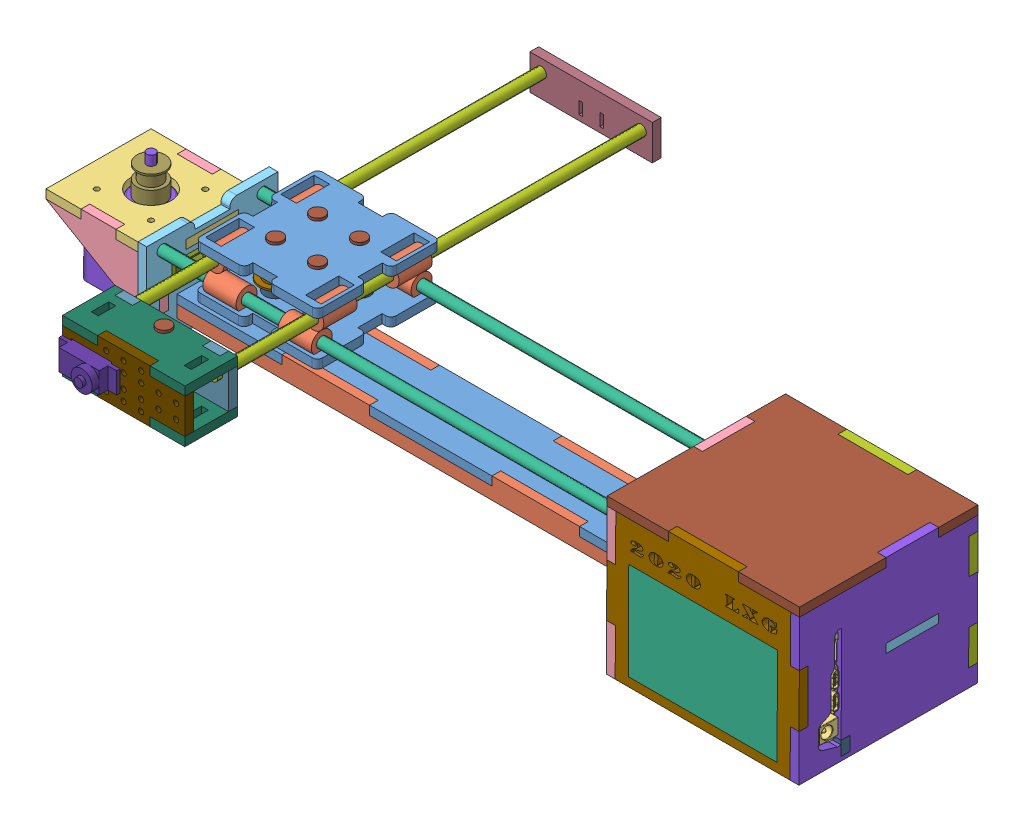
SolidWorks assembly 合V1.0, configuration 默认. Lengths in mm.
Overall size (465 88.44 285.26).
63 component instances, 29 part files, 128 mates.
Components (placement in the parent):
- 中心同步块-1: 中心同步块 [默认] at (-116.6311 89.0687 -129.5565) x (0 0.004224 0.999991) z (0 -0.999991 0.004224) size (70 70 5)
- 中心同步块-2: 中心同步块 [默认] at (-186.6311 114.1177 -129.6623) x (1 0 0) z (0 -0.999991 0.004224) size (70 70 5)
- 直线轴承 内径6MMx外径12MMx长度19MM-1: 直线轴承 内径6MMx外径12MMx长度19MM [默认] at (-139.6311 93.3617 -66.024) x (0 0.863153 -0.504943) z (1 0 0) size (13.89 12 19)
- 直线轴承 内径6MMx外径12MMx长度19MM-2: 直线轴承 内径6MMx外径12MMx长度19MM [默认] at (-180.1811 105.1903 -106.6244) x (0.934679 0.35549 -0.001501) z (0 -0.004224 -0.999991) size (13.89 12 19)
- 长端无控制器端电机座上-1: 长端无控制器端电机座上 [默认] at (-216.7731 91.6144 -124.5672) x (0 0.004224 0.999991) z (0 -0.999991 0.004224) size (60 65 5)
- 长端无控制器端电机座侧面-1: 长端无控制器端电机座侧面 [默认] at (-216.7731 51.8471 -69.3987) x (1 0 0) z (0 0.004224 0.999991) size (65 40 5)
- 长端无控制器端电机座侧面-2: 长端无控制器端电机座侧面 [默认] at (-216.7731 51.6148 -124.3982) x (1 0 0) z (0 0.004224 0.999991) size (65 40 5)
- 长端无控制器端-1: 长端无控制器端 [默认] at (-216.7731 46.0726 -134.3749) x (0 -0.004224 -0.999991) z (1 0 0) size (80 53 5)
- 直线轴承 内径6MMx外径12MMx长度19MM-3: 直线轴承 内径6MMx外径12MMx长度19MM [默认] at (-182.6311 93.1205 -123.1235) x (0 0.999978 -0.006661) z (1 0 0) size (13.89 12 19)
- 直线轴承 内径6MMx外径12MMx长度19MM-4: 直线轴承 内径6MMx外径12MMx长度19MM [默认] at (-182.6311 93.3617 -66.024) x (0 0.949917 -0.312502) z (1 0 0) size (13.89 12 19)
- 直线轴承 内径6MMx外径12MMx长度19MM-5: 直线轴承 内径6MMx外径12MMx长度19MM [默认] at (-139.6311 93.1205 -123.1235) x (0 0.946256 0.323419) z (1 0 0) size (13.89 12 19)
- 直线轴承 内径6MMx外径12MMx长度19MM-6: 直线轴承 内径6MMx外径12MMx长度19MM [默认] at (-123.0811 105.2917 -82.6246) x (-0.725747 -0.687956 0.002906) z (0 0.004224 0.999991) size (13.89 12 19)
- 直线轴承 内径6MMx外径12MMx长度19MM-7: 直线轴承 内径6MMx外径12MMx长度19MM [默认] at (-123.0811 105.1903 -106.6244) x (1 0 0) z (0 -0.004224 -0.999991) size (13.89 12 19)
- 直线轴承 内径6MMx外径12MMx长度19MM-8: 直线轴承 内径6MMx外径12MMx长度19MM [默认] at (-180.1811 105.3719 -63.6247) x (1 0 0) z (0 -0.004224 -0.999991) size (13.89 12 19)
- 光杆300MMx6MM-1: 光杆300MMx6MM [默认] at (83.2269 93.3617 -66.024) x (0 0 1) z (-1 0 0) size (6 6 300)
- 光杆300MMx6MM-2: 光杆300MMx6MM [默认] at (83.2269 93.1205 -123.1235) x (0 0 1) z (-1 0 0) size (6 6 300)
- 光杆250MMx6MM-3: 光杆250MMx6MM [默认] at (-180.1811 104.5595 -255.9817) x (-0.383385 -0.92358 0.003901) z (0 0.004224 0.999991) size (6 6 250)
- 光杆250MMx6MM-4: 光杆250MMx6MM [默认] at (-123.0811 104.5595 -255.9817) x (0.573262 0.819365 -0.003461) z (0 0.004224 0.999991) size (6 6 250)
- 42步进电机-1: 42步进电机 [默认] at (-267.9231 86.8305 -73.3965) x (0 -0.999991 0.004224) z (0 0.004224 0.999991) size (61.5 49.3 42.3)
- 42步进电机-2: 42步进电机 [默认] at (134.3769 86.6518 -115.6961) x (0 -0.999991 0.004224) z (0 -0.004224 -0.999991) size (61.5 49.3 42.3)
- 2GT_20齿同步轮 H型皮带轮 带宽6MM 内孔5MM-1: 2GT_20齿同步轮 H型皮带轮 带宽6MM 内孔5MM [默认] at (-163.6311 102.4606 -82.6126) x (0.996537 0.000351 0.08315) z (0 -0.999991 0.004224) size (18 18 8.5)
- 内径5MM 外径10MM 厚度6MM隔离柱-1: 内径5MM 外径10MM 厚度6MM隔离柱 [默认] at (-163.6311 103.4606 -82.6168) x (1 0 0) z (0 0.004224 0.999991) size (12 6 12)
- M5x35MM螺丝-1: M5x35MM螺丝 [默认] at (-163.6311 79.3165 -82.5149) x (1 0 0) z (0 0.004224 0.999991) size (8.05 36.5 8.05)
- 内径5MM 外径10MM 厚度6MM隔离柱-2: 内径5MM 外径10MM 厚度6MM隔离柱 [默认] at (-163.6311 88.9607 -82.5556) x (1 0 0) z (0 0.004224 0.999991) size (12 6 12)
- 内径5MM 外径10MM 厚度6MM隔离柱-3: 内径5MM 外径10MM 厚度6MM隔离柱 [默认] at (-139.6311 107.2087 -82.6327) x (0.081874 0.004209 0.996634) z (-0.996643 0.000346 0.081873) size (12 6 12)
- 2GT_20齿同步轮 H型皮带轮 带宽6MM 内孔5MM-2: 2GT_20齿同步轮 H型皮带轮 带宽6MM 内孔5MM [默认] at (-139.6311 106.2087 -82.6284) x (1 0 0) z (0 -0.999991 0.004224) size (18 18 8.5)
- 内径5MM 外径10MM 厚度6MM隔离柱-4: 内径5MM 外径10MM 厚度6MM隔离柱 [默认] at (-139.6311 92.7089 -82.5714) x (0.998633 -0.000221 -0.052265) z (0.052266 0.004218 0.998624) size (12 6 12)
- M5x35MM螺丝-2: M5x35MM螺丝 [默认] at (-139.6311 79.3165 -82.5149) x (1 0 0) z (0 0.004224 0.999991) size (8.05 36.5 8.05)
- 同步轮2GT带宽6MM 20齿内孔5MM-1: 同步轮2GT带宽6MM 20齿内孔5MM [默认] at (-246.7731 88.7411 -94.5548) x (0.755628 0.002766 0.654995) z (-0.655001 0.003191 0.755621) size (16 16 16)
- 内径5MM 外径10MM 厚度6MM隔离柱-5: 内径5MM 外径10MM 厚度6MM隔离柱 [默认] at (-163.6311 89.4064 -106.5577) x (1 0 0) z (0 0.004224 0.999991) size (12 6 12)
- M5x35MM螺丝-3: M5x35MM螺丝 [默认] at (-163.6311 79.2152 -106.5146) x (1 0 0) z (0 0.004224 0.999991) size (8.05 36.5 8.05)
- 2GT_20齿同步轮 H型皮带轮 带宽6MM 内孔5MM-3: 2GT_20齿同步轮 H型皮带轮 带宽6MM 内孔5MM [默认] at (-163.6311 102.9063 -106.6147) x (1 0 0) z (0 -0.999991 0.004224) size (18 18 8.5)
- 内径5MM 外径10MM 厚度6MM隔离柱-6: 内径5MM 外径10MM 厚度6MM隔离柱 [默认] at (-163.6311 103.9063 -106.6189) x (0.113852 0.004196 0.993489) z (-0.993498 0.000481 0.113851) size (12 6 12)
- 内径5MM 外径10MM 厚度6MM隔离柱-7: 内径5MM 外径10MM 厚度6MM隔离柱 [默认] at (-139.6311 89.407 -106.5577) x (0.997535 -0.000296 -0.070166) z (0.070166 0.004213 0.997526) size (12 6 12)
- M5x35MM螺丝-4: M5x35MM螺丝 [默认] at (-139.6311 79.2152 -106.5146) x (1 0 0) z (0 0.004224 0.999991) size (8.05 36.5 8.05)
- 2GT_20齿同步轮 H型皮带轮 带宽6MM 内孔5MM-4: 2GT_20齿同步轮 H型皮带轮 带宽6MM 内孔5MM [默认] at (-139.6311 102.9069 -106.6147) x (1 0 0) z (0 -0.999991 0.004224) size (18 18 8.5)
- 内径5MM 外径10MM 厚度6MM隔离柱-8: 内径5MM 外径10MM 厚度6MM隔离柱 [默认] at (-139.6311 103.9069 -106.6189) x (0.631814 0.003274 0.775113) z (-0.77512 0.002669 0.631809) size (12 6 12)
- 短端结扎-1: 短端结扎 [默认] at (-151.6311 101.5595 -255.9691) x (1 0 0) z (0 -0.999991 0.004224) size (70 5 20)
- 短端抬笔侧-1: 短端抬笔侧 [默认] at (-186.6311 89.5825 -13.7378) x (1 0 0) z (0 -0.999991 0.004224) size (20 5 30)
- 短端抬笔上-1: 短端抬笔上 [默认] at (-186.6311 109.709 16.1774) x (1 0 0) z (0 0.004224 0.999991) size (70 5 30)
- 短端抬笔侧-2: 短端抬笔侧 [默认] at (-116.6311 89.6036 -8.7379) x (-1 0 0) z (0 -0.999991 0.004224) size (20 5 30)
- 短端抬笔上-2: 短端抬笔上 [默认] at (-116.6311 89.7092 16.2619) x (-1 0 0) z (0 0.004224 0.999991) size (70 5 30)
- M5x35MM螺丝-5: M5x35MM螺丝 [默认] at (-151.6311 79.6121 -6.6957) x (-0.916947 0.001685 0.399005) z (-0.399008 -0.003873 -0.916939) size (8.05 36.5 8.05)
- 内径5MM 外径10MM 厚度6MM隔离柱-9: 内径5MM 外径10MM 厚度6MM隔离柱 [默认] at (-151.6311 89.2051 -6.7362) x (0.998633 -0.000221 -0.052265) z (0.052266 0.004218 0.998624) size (12 6 12)
- 2GT_20齿同步轮 H型皮带轮 带宽6MM 内孔5MM-5: 2GT_20齿同步轮 H型皮带轮 带宽6MM 内孔5MM [默认] at (-151.6311 102.705 -6.7932) x (1 0 0) z (0 -0.999991 0.004224) size (18 18 8.5)
- 内径5MM 外径10MM 厚度6MM隔离柱-10: 内径5MM 外径10MM 厚度6MM隔离柱 [默认] at (-151.6311 103.705 -6.7974) x (0.928854 0.001565 0.370443) z (-0.370447 0.003923 0.928845) size (12 6 12)
- 限位开关-1: 限位开关 [默认] at (-225.4635 76.6652 -112.5039) x (0 0.004224 0.999991) z (-1 0 0) size (41 7.3 21.5)
- SG90舵机-1: SG90舵机 [默认] at (-181.6311 92.7091 1.2491) x (1 0 0) z (0 -0.999991 0.004224) size (33 28 12.05)
- 短端抬笔前-1: 短端抬笔前 [默认] at (-186.6311 89.6881 11.2619) x (1 0 0) z (0 -0.999991 0.004224) size (70 5 30)
- 底部大横-1: 底部大横 [默认] at (-211.7731 62.1569 -114.4427) x (0 0.004224 0.999991) z (-1 0 0) size (40 5 300)
- 底部大横竖-1: 底部大横竖 [默认] at (-216.7731 55.3048 -79.4134) x (1 0 0) z (0 -0.999991 0.004224) size (300 5 12)
- 底部大横竖-2: 底部大横竖 [默认] at (-216.7731 55.157 -114.4131) x (1 0 0) z (0 -0.999991 0.004224) size (300 5 12)
- 限位开关-2: 限位开关 [默认] at (-145.6311 84.6501 2.2831) x (-1 0 0) z (0 0.004224 0.999991) size (41 7.3 21.5)
- ArtistV1-1: ArtistV1 [默认] at (88.2308 47.6829 -53.5734) x (1 0 0) z (0 0.004224 0.999991) size (99.16 80.01 19.91)
- 长端控制器端-1: 长端控制器端 [默认] at (83.2269 46.4105 -54.3756) x (0 0.004224 0.999991) z (-1 0 0) size (102 88 5)
- 长端控制器端电机座上-1: 长端控制器端电机座上 [默认] at (83.2269 86.6144 -124.5461) x (0 0.004224 0.999991) z (0 0.999991 -0.004224) size (62.5 110 5)
- 同步轮2GT带宽6MM 20齿内孔5MM-2: 同步轮2GT带宽6MM 20齿内孔5MM [默认] at (113.2269 92.1104 -94.569) x (0.99941 -0.000145 -0.034342) z (0.034343 0.004221 0.999401) size (16 16 16)
- 3.5寸LCD-1: 3.5寸LCD [默认] at (37.2293 48.6901 -33.4851) x (1 0 0) z (0 0.004224 0.999991) size (85 55.5 3.6)
- 长端控制器端后-1: 长端控制器端后 [默认] at (83.2269 46.0831 -131.8749) x (1 0 0) z (0 0.004224 0.999991) size (110 88 5)
- 长端控制器端右-1: 长端控制器端右 [默认] at (188.2269 76.8541 -60.2099) x (-1 0 0) z (0 -0.004224 -0.999991) size (5 88 102)
- 长端控制器端前-1: 长端控制器端前 [默认] at (83.2269 46.4928 -34.8758) x (1 0 0) z (0 0.004224 0.999991) size (110 88 5)
- 长端控制器端pcb座-1: 长端控制器端pcb座 [默认] at (157.8191 48.8702 -53.9544) x (0 -0.004224 -0.999991) z (1 0 0) size (5 20 110)
- 长端控制器端上-1: 长端控制器端上 [默认] at (78.2269 129.5132 -30.2264) x (1 0 0) z (0 0.004224 0.999991) size (110 5 102)
Mates (geometry in assembly coordinates):
- 重合1: coincident aligned: line of 长端无控制器端电机座上-1 through (-211.7731 91.6778 -109.5673) axis (0 0.004224 0.999991); line of 长端无控制器端-1 through (-211.7731 91.6778 -109.5673) axis (0 0.004224 0.999991)
- 重合2: coincident anti-aligned: line of 长端无控制器端电机座上-1 through (-211.7731 86.8045 -79.5465) axis (0 0.999991 -0.004224); line of 长端无控制器端-1 through (-211.7731 91.8045 -79.5676) axis (0 -0.999991 0.004224)
- 重合3: coincident aligned: line of 长端无控制器端电机座上-1 through (-236.7731 91.8467 -69.5677) axis (-1 0 0); line of 长端无控制器端电机座侧面-1 through (-236.7731 91.8467 -69.5677) axis (-1 0 0)
- 重合4: coincident aligned: line of 长端无控制器端电机座上-1 through (-236.7731 91.8678 -64.5677) axis (0 -0.004224 -0.999991); line of 长端无控制器端电机座侧面-1 through (-236.7731 91.8678 -64.5677) axis (0 -0.004224 -0.999991)
- 重合5: coincident anti-aligned: line of 长端无控制器端电机座上-1 through (-256.7731 91.6355 -119.5672) axis (1 0 0); line of 长端无控制器端电机座侧面-2 through (-236.7731 91.6355 -119.5672) axis (-1 0 0)
- 重合6: coincident aligned: line of 长端无控制器端电机座上-1 through (-236.7731 91.6355 -119.5672) axis (0 -0.004224 -0.999991); line of 长端无控制器端电机座侧面-2 through (-236.7731 91.6355 -119.5672) axis (0 -0.004224 -0.999991)
- 重合13: coincident anti-aligned: circle of 长端无控制器端电机座上-1; circle of 42步进电机-1
- 同心1: concentric anti-aligned: cylinder of 长端无控制器端-1 through (-211.7731 93.3617 -66.024) axis (-1 0 0) radius 3; cylinder of 光杆300MMx6MM-1 through (-216.7731 93.3617 -66.024) axis (1 0 0) radius 3
- 同心2: concentric anti-aligned: cylinder of 长端无控制器端-1 through (-211.7731 93.1205 -123.1235) axis (-1 0 0) radius 3; cylinder of 光杆300MMx6MM-2 through (-216.7731 93.1205 -123.1235) axis (1 0 0) radius 3
- 重合17: coincident anti-aligned: circle of 长端无控制器端-1; circle of 光杆300MMx6MM-1
- 重合18: coincident anti-aligned: circle of 长端无控制器端-1; circle of 光杆300MMx6MM-2
- 同心6: concentric anti-aligned: cylinder of 直线轴承 内径6MMx外径12MMx长度19MM-4 through (-163.6311 93.3617 -66.024) axis (-1 0 0) radius 3; cylinder of 光杆300MMx6MM-1 through (-216.7731 93.3617 -66.024) axis (1 0 0) radius 3
- 同心7: concentric anti-aligned: cylinder of 直线轴承 内径6MMx外径12MMx长度19MM-1 through (-120.6311 93.3617 -66.024) axis (-1 0 0) radius 3; cylinder of 光杆300MMx6MM-1 through (-216.7731 93.3617 -66.024) axis (1 0 0) radius 3
- 同心8: concentric anti-aligned: cylinder of 直线轴承 内径6MMx外径12MMx长度19MM-3 through (-163.6311 93.1205 -123.1235) axis (-1 0 0) radius 3; cylinder of 光杆300MMx6MM-2 through (-216.7731 93.1205 -123.1235) axis (1 0 0) radius 3
- 同心9: concentric anti-aligned: cylinder of 直线轴承 内径6MMx外径12MMx长度19MM-5 through (-120.6311 93.1205 -123.1235) axis (-1 0 0) radius 3; cylinder of 光杆300MMx6MM-2 through (-216.7731 93.1205 -123.1235) axis (1 0 0) radius 3
- 同心10: concentric anti-aligned: cylinder of 2GT_20齿同步轮 H型皮带轮 带宽6MM 内孔5MM-1 through (-163.6311 95.9606 -82.5852) axis (0 0.999991 -0.004224) radius 2.5; cylinder of M5x35MM螺丝-1 through (-163.6311 114.3162 -82.6627) axis (0 -0.999991 0.004224) radius 2.5
- 同心11: concentric aligned: cylinder of 内径5MM 外径10MM 厚度6MM隔离柱-1 through (-163.6311 109.4605 -82.6422) axis (0 -0.999991 0.004224) radius 3; cylinder of M5x35MM螺丝-1 through (-163.6311 114.3162 -82.6627) axis (0 -0.999991 0.004224) radius 2.5
- 同心12: concentric aligned: cylinder of M5x35MM螺丝-1 through (-163.6311 114.3162 -82.6627) axis (0 -0.999991 0.004224) radius 2.5; cylinder of 内径5MM 外径10MM 厚度6MM隔离柱-2 through (-163.6311 94.9607 -82.5809) axis (0 -0.999991 0.004224) radius 3
- 同心13: concentric aligned: cylinder of 内径5MM 外径10MM 厚度6MM隔离柱-3 through (-139.6311 113.2087 -82.658) axis (0 -0.999991 0.004224) radius 3; cylinder of M5x35MM螺丝-2 through (-139.6311 114.3162 -82.6627) axis (0 -0.999991 0.004224) radius 2.5
- 同心14: concentric aligned: cylinder of 内径5MM 外径10MM 厚度6MM隔离柱-4 through (-139.6311 98.7088 -82.5968) axis (0 -0.999991 0.004224) radius 3; cylinder of M5x35MM螺丝-2 through (-139.6311 114.3162 -82.6627) axis (0 -0.999991 0.004224) radius 2.5
- 同心15: concentric anti-aligned: cylinder of 2GT_20齿同步轮 H型皮带轮 带宽6MM 内孔5MM-2 through (-139.6311 99.7088 -82.601) axis (0 0.999991 -0.004224) radius 2.5; cylinder of M5x35MM螺丝-2 through (-139.6311 114.3162 -82.6627) axis (0 -0.999991 0.004224) radius 2.5
- 重合19: coincident aligned: plane of 2GT_20齿同步轮 H型皮带轮 带宽6MM 内孔5MM-1 through (-163.6311 103.4606 -82.6168) normal (0 0.999991 -0.004224); circle of 内径5MM 外径10MM 厚度6MM隔离柱-1
- 重合20: coincident anti-aligned: plane of 2GT_20齿同步轮 H型皮带轮 带宽6MM 内孔5MM-1 through (-163.6311 94.9607 -82.5809) normal (0 -0.999991 0.004224); plane of 内径5MM 外径10MM 厚度6MM隔离柱-2 through (-163.6311 94.9607 -82.5809) normal (0 0.999991 -0.004224)
- 同心16: concentric aligned: cylinder of 中心同步块-1 through (-163.6311 84.2673 -82.5358) axis (0 0.999991 -0.004224) radius 2.5; cylinder of 中心同步块-2 through (-163.6311 109.3163 -82.6416) axis (0 0.999991 -0.004224) radius 2.5
- 同心17: concentric aligned: cylinder of 中心同步块-1 through (-139.6311 84.2673 -82.5358) axis (0 0.999991 -0.004224) radius 2.5; cylinder of 中心同步块-2 through (-139.6311 109.3163 -82.6416) axis (0 0.999991 -0.004224) radius 2.5
- 同心18: concentric anti-aligned: cylinder of 中心同步块-2 through (-163.6311 109.3163 -82.6416) axis (0 0.999991 -0.004224) radius 2.5; cylinder of M5x35MM螺丝-1 through (-163.6311 114.3162 -82.6627) axis (0 -0.999991 0.004224) radius 2.5
- 重合21: coincident anti-aligned: plane of 中心同步块-2 through (-161.6311 114.1304 -126.6623) normal (0 0.999991 -0.004224); plane of M5x35MM螺丝-1 through (-163.6311 114.3162 -82.6627) normal (0 -0.999991 0.004224)
- 相切2: tangent: line of 中心同步块-1 through (-163.6311 89.1147 -118.6566) axis (-1 0 0); cylinder of 直线轴承 内径6MMx外径12MMx长度19MM-3 through (-163.6311 93.1205 -123.1235) axis (-1 0 0) radius 6
- 重合24: coincident: line of 中心同步块-1 through (-182.6311 89.3559 -61.5571) axis (0 -0.004224 -0.999991); plane of 直线轴承 内径6MMx外径12MMx长度19MM-4 through (-182.6311 93.3617 -66.024) normal (-1 0 0)
- 重合25: coincident: line of 中心同步块-1 through (-163.6311 89.3559 -61.5571) axis (-1 0 0); cylinder of 直线轴承 内径6MMx外径12MMx长度19MM-4 through (-163.6311 93.3617 -66.024) axis (-1 0 0) radius 6
- 重合26: coincident: line of 中心同步块-1 through (-182.6311 89.1147 -118.6566) axis (0 -0.004224 -0.999991); plane of 直线轴承 内径6MMx外径12MMx长度19MM-3 through (-182.6311 93.1205 -123.1235) normal (-1 0 0)
- 重合27: coincident: line of 中心同步块-1 through (-182.6311 89.3183 -70.457) axis (1 0 0); cylinder of 直线轴承 内径6MMx外径12MMx长度19MM-4 through (-163.6311 93.3617 -66.024) axis (-1 0 0) radius 6
- 重合28: coincident: line of 中心同步块-1 through (-120.6311 89.3183 -70.457) axis (0 0.004224 0.999991); plane of 直线轴承 内径6MMx外径12MMx长度19MM-1 through (-120.6311 93.3617 -66.024) normal (1 0 0)
- 重合29: coincident: line of 中心同步块-1 through (-120.6311 89.0771 -127.5565) axis (0 0.004224 0.999991); plane of 直线轴承 内径6MMx外径12MMx长度19MM-5 through (-120.6311 93.1205 -123.1235) normal (1 0 0)
- 重合30: coincident: line of 中心同步块-2 through (-184.6311 109.3965 -63.6417) axis (0 -0.004224 -0.999991); cylinder of 直线轴承 内径6MMx外径12MMx长度19MM-8 through (-180.1811 105.2917 -82.6246) axis (0 0.004224 0.999991) radius 6
- 重合31: coincident: line of 中心同步块-2 through (-175.7311 109.3163 -82.6416) axis (0 0.004224 0.999991); cylinder of 直线轴承 内径6MMx外径12MMx长度19MM-8 through (-180.1811 105.2917 -82.6246) axis (0 0.004224 0.999991) radius 6
- 重合32: coincident anti-aligned: plane of 中心同步块-2 through (-184.6311 109.3163 -82.6416) normal (0 0.004224 0.999991); plane of 直线轴承 内径6MMx外径12MMx长度19MM-8 through (-180.1811 105.2917 -82.6246) normal (0 -0.004224 -0.999991)
- 相切3: tangent anti-aligned: cylinder of 直线轴承 内径6MMx外径12MMx长度19MM-4 through (-163.6311 93.3617 -66.024) axis (-1 0 0) radius 6; cylinder of 直线轴承 内径6MMx外径12MMx长度19MM-8 through (-180.1811 105.2917 -82.6246) axis (0 0.004224 0.999991) radius 6
- 同心20: concentric anti-aligned: cylinder of 直线轴承 内径6MMx外径12MMx长度19MM-8 through (-180.1811 105.2917 -82.6246) axis (0 0.004224 0.999991) radius 3; cylinder of 光杆250MMx6MM-3 through (-180.1811 105.6154 -5.984) axis (0 -0.004224 -0.999991) radius 3
- 重合33: coincident anti-aligned: plane of 中心同步块-2 through (-127.5311 109.3163 -82.6416) normal (0 0.004224 0.999991); plane of 直线轴承 内径6MMx外径12MMx长度19MM-6 through (-123.0811 105.2917 -82.6246) normal (0 -0.004224 -0.999991)
- 重合36: coincident: line of 中心同步块-2 through (-118.6311 109.3163 -82.6416) axis (0 0.004224 0.999991); cylinder of 直线轴承 内径6MMx外径12MMx长度19MM-6 through (-123.0811 105.3719 -63.6247) axis (0 -0.004224 -0.999991) radius 6
- 重合37: coincident: line of 中心同步块-2 through (-127.5311 109.3965 -63.6417) axis (0 -0.004224 -0.999991); cylinder of 直线轴承 内径6MMx外径12MMx长度19MM-6 through (-123.0811 105.3719 -63.6247) axis (0 -0.004224 -0.999991) radius 6
- 重合38: coincident: line of 中心同步块-2 through (-127.5311 109.2149 -106.6414) axis (0 -0.004224 -0.999991); cylinder of 直线轴承 内径6MMx外径12MMx长度19MM-7 through (-123.0811 105.1101 -125.6242) axis (0 0.004224 0.999991) radius 6
- 重合39: coincident: line of 中心同步块-2 through (-118.6311 109.1346 -125.6412) axis (0 0.004224 0.999991); cylinder of 直线轴承 内径6MMx外径12MMx长度19MM-7 through (-123.0811 105.1101 -125.6242) axis (0 0.004224 0.999991) radius 6
- 重合40: coincident anti-aligned: plane of 中心同步块-2 through (-127.5311 109.1346 -125.6412) normal (0 0.004224 0.999991); plane of 直线轴承 内径6MMx外径12MMx长度19MM-7 through (-123.0811 105.1101 -125.6242) normal (0 -0.004224 -0.999991)
- 重合43: coincident anti-aligned: plane of 中心同步块-2 through (-184.6311 109.2149 -106.6414) normal (0 -0.004224 -0.999991); plane of 直线轴承 内径6MMx外径12MMx长度19MM-2 through (-180.1811 105.1903 -106.6244) normal (0 0.004224 0.999991)
- 相切4: tangent anti-aligned: cylinder of 直线轴承 内径6MMx外径12MMx长度19MM-2 through (-180.1811 105.1101 -125.6242) axis (0 0.004224 0.999991) radius 6; cylinder of 直线轴承 内径6MMx外径12MMx长度19MM-3 through (-163.6311 93.1205 -123.1235) axis (-1 0 0) radius 6
- 同心21: concentric aligned: cylinder of 直线轴承 内径6MMx外径12MMx长度19MM-6 through (-123.0811 105.3719 -63.6247) axis (0 -0.004224 -0.999991) radius 3; cylinder of 光杆250MMx6MM-4 through (-123.0811 105.6154 -5.984) axis (0 -0.004224 -0.999991) radius 3
- 重合44: coincident: line of 中心同步块-2 through (-175.7311 109.1346 -125.6412) axis (0 0.004224 0.999991); cylinder of 直线轴承 内径6MMx外径12MMx长度19MM-2 through (-180.1811 105.1101 -125.6242) axis (0 0.004224 0.999991) radius 6
- 同心22: concentric aligned: cylinder of 42步进电机-1 through (-246.7731 110.2409 -94.6456) axis (0 -0.999991 0.004224) radius 2.5; cylinder of 同步轮2GT带宽6MM 20齿内孔5MM-1 through (-246.7731 96.7411 -94.5886) axis (0 -0.999991 0.004224) radius 2.5
- 重合45: coincident anti-aligned: circle of 长端无控制器端电机座上-1; circle of 42步进电机-1
- 重合46: coincident anti-aligned: plane of 42步进电机-1 through (-246.7731 88.7411 -94.5548) normal (0 0.999991 -0.004224); plane of 同步轮2GT带宽6MM 20齿内孔5MM-1 through (-246.7731 88.7411 -94.5548) normal (0 -0.999991 0.004224)
- 重合47: coincident anti-aligned: plane of 内径5MM 外径10MM 厚度6MM隔离柱-3 through (-139.6311 107.2087 -82.6327) normal (0 -0.999991 0.004224); plane of 2GT_20齿同步轮 H型皮带轮 带宽6MM 内孔5MM-2 through (-139.6311 107.2087 -82.6327) normal (0 0.999991 -0.004224)
- 重合48: coincident anti-aligned: plane of 2GT_20齿同步轮 H型皮带轮 带宽6MM 内孔5MM-2 through (-139.6311 98.7088 -82.5968) normal (0 -0.999991 0.004224); plane of 内径5MM 外径10MM 厚度6MM隔离柱-4 through (-139.6311 98.7088 -82.5968) normal (0 0.999991 -0.004224)
- 同心23: concentric anti-aligned: cylinder of 中心同步块-2 through (-139.6311 109.3163 -82.6416) axis (0 0.999991 -0.004224) radius 2.5; cylinder of M5x35MM螺丝-2 through (-139.6311 114.3162 -82.6627) axis (0 -0.999991 0.004224) radius 2.5
- 同心24: concentric aligned: cylinder of 内径5MM 外径10MM 厚度6MM隔离柱-5 through (-163.6311 95.4064 -106.583) axis (0 -0.999991 0.004224) radius 3; cylinder of M5x35MM螺丝-3 through (-163.6311 114.2148 -106.6625) axis (0 -0.999991 0.004224) radius 2.5
- 同心25: concentric aligned: cylinder of M5x35MM螺丝-3 through (-163.6311 114.2148 -106.6625) axis (0 -0.999991 0.004224) radius 2.5; cylinder of 内径5MM 外径10MM 厚度6MM隔离柱-6 through (-163.6311 109.9063 -106.6443) axis (0 -0.999991 0.004224) radius 3
- 同心26: concentric anti-aligned: cylinder of M5x35MM螺丝-3 through (-163.6311 114.2148 -106.6625) axis (0 -0.999991 0.004224) radius 2.5; cylinder of 2GT_20齿同步轮 H型皮带轮 带宽6MM 内孔5MM-3 through (-163.6311 96.4064 -106.5873) axis (0 0.999991 -0.004224) radius 2.5
- 重合49: coincident anti-aligned: plane of 内径5MM 外径10MM 厚度6MM隔离柱-5 through (-163.6311 95.4064 -106.583) normal (0 0.999991 -0.004224); plane of 2GT_20齿同步轮 H型皮带轮 带宽6MM 内孔5MM-3 through (-163.6311 95.4064 -106.583) normal (0 -0.999991 0.004224)
- 重合50: coincident anti-aligned: plane of 2GT_20齿同步轮 H型皮带轮 带宽6MM 内孔5MM-3 through (-163.6311 103.9063 -106.6189) normal (0 0.999991 -0.004224); plane of 内径5MM 外径10MM 厚度6MM隔离柱-6 through (-163.6311 103.9063 -106.6189) normal (0 -0.999991 0.004224)
- 同心27: concentric aligned: cylinder of 内径5MM 外径10MM 厚度6MM隔离柱-7 through (-139.6311 95.407 -106.583) axis (0 -0.999991 0.004224) radius 3; cylinder of M5x35MM螺丝-4 through (-139.6311 114.2148 -106.6625) axis (0 -0.999991 0.004224) radius 2.5
- 同心28: concentric aligned: cylinder of M5x35MM螺丝-4 through (-139.6311 114.2148 -106.6625) axis (0 -0.999991 0.004224) radius 2.5; cylinder of 内径5MM 外径10MM 厚度6MM隔离柱-8 through (-139.6311 109.9069 -106.6443) axis (0 -0.999991 0.004224) radius 3
- 同心29: concentric anti-aligned: cylinder of M5x35MM螺丝-4 through (-139.6311 114.2148 -106.6625) axis (0 -0.999991 0.004224) radius 2.5; cylinder of 2GT_20齿同步轮 H型皮带轮 带宽6MM 内孔5MM-4 through (-139.6311 96.407 -106.5873) axis (0 0.999991 -0.004224) radius 2.5
- 重合51: coincident anti-aligned: plane of 内径5MM 外径10MM 厚度6MM隔离柱-7 through (-139.6311 95.407 -106.583) normal (0 0.999991 -0.004224); plane of 2GT_20齿同步轮 H型皮带轮 带宽6MM 内孔5MM-4 through (-139.6311 95.407 -106.583) normal (0 -0.999991 0.004224)
- 重合52: coincident anti-aligned: plane of 2GT_20齿同步轮 H型皮带轮 带宽6MM 内孔5MM-4 through (-139.6311 103.9069 -106.6189) normal (0 0.999991 -0.004224); plane of 内径5MM 外径10MM 厚度6MM隔离柱-8 through (-139.6311 103.9069 -106.6189) normal (0 -0.999991 0.004224)
- 同心30: concentric anti-aligned: cylinder of 中心同步块-2 through (-163.6311 109.2149 -106.6414) axis (0 0.999991 -0.004224) radius 2.5; cylinder of M5x35MM螺丝-3 through (-163.6311 114.2148 -106.6625) axis (0 -0.999991 0.004224) radius 2.5
- 同心31: concentric anti-aligned: cylinder of 中心同步块-2 through (-139.6311 109.2149 -106.6414) axis (0 0.999991 -0.004224) radius 2.5; cylinder of M5x35MM螺丝-4 through (-139.6311 114.2148 -106.6625) axis (0 -0.999991 0.004224) radius 2.5
- 重合53: coincident aligned: plane of 中心同步块-2 through (-161.6311 114.1304 -126.6623) normal (0 0.999991 -0.004224); circle of M5x35MM螺丝-2
- 重合54: coincident aligned: plane of 中心同步块-2 through (-161.6311 114.1304 -126.6623) normal (0 0.999991 -0.004224); circle of M5x35MM螺丝-3
- 重合55: coincident aligned: plane of 中心同步块-2 through (-161.6311 114.1304 -126.6623) normal (0 0.999991 -0.004224); circle of M5x35MM螺丝-4
- 同心32: concentric aligned: cylinder of 光杆250MMx6MM-3 through (-180.1811 105.6154 -5.984) axis (0 -0.004224 -0.999991) radius 3; cylinder of 短端结扎-1 through (-180.1811 104.5806 -250.9818) axis (0 -0.004224 -0.999991) radius 3
- 同心33: concentric aligned: cylinder of 光杆250MMx6MM-4 through (-123.0811 105.6154 -5.984) axis (0 -0.004224 -0.999991) radius 3; cylinder of 短端结扎-1 through (-123.0811 104.5806 -250.9818) axis (0 -0.004224 -0.999991) radius 3
- 重合56: coincident aligned: circle of 光杆250MMx6MM-3; circle of 短端结扎-1
- 重合57: coincident aligned: circle of 光杆250MMx6MM-4; circle of 短端结扎-1
- 锁定1: lock: unknown of 中心同步块-2; unknown of 直线轴承 内径6MMx外径12MMx长度19MM-6
- 重合58: coincident aligned: line of 短端抬笔侧-1 through (-171.6311 114.6034 -8.8435) axis (-1 0 0); line of 短端抬笔上-1 through (-171.6311 114.6034 -8.8435) axis (-1 0 0)
- 重合59: coincident aligned: line of 短端抬笔侧-1 through (-181.6311 114.6034 -8.8435) axis (0 -0.004224 -0.999991); line of 短端抬笔上-1 through (-181.6311 114.6034 -8.8435) axis (0 -0.004224 -0.999991)
- 重合63: coincident anti-aligned: line of 短端抬笔上-1 through (-131.6311 114.6034 -8.8435) axis (0 -0.004224 -0.999991); line of 短端抬笔侧-2 through (-131.6311 114.5823 -13.8434) axis (0 0.004224 0.999991)
- 重合64: coincident anti-aligned: line of 短端抬笔上-1 through (-121.6311 114.6034 -8.8435) axis (-1 0 0); line of 短端抬笔侧-2 through (-131.6311 114.6034 -8.8435) axis (1 0 0)
- 重合65: coincident aligned: line of 短端抬笔侧-1 through (-181.6311 84.6036 -8.7168) axis (1 0 0); line of 短端抬笔上-2 through (-181.6311 84.6036 -8.7168) axis (1 0 0)
- 重合66: coincident aligned: line of 短端抬笔侧-1 through (-171.6311 84.6036 -8.7168) axis (0 0.999991 -0.004224); line of 短端抬笔上-2 through (-171.6311 84.6036 -8.7168) axis (0 0.999991 -0.004224)
- 同心34: concentric aligned: cylinder of 光杆250MMx6MM-3 through (-180.1811 105.6154 -5.984) axis (0 -0.004224 -0.999991) radius 3; cylinder of 短端抬笔侧-1 through (-180.1811 105.6035 -8.8055) axis (0 -0.004224 -0.999991) radius 3
- 同心35: concentric anti-aligned: cylinder of 光杆250MMx6MM-4 through (-123.0811 105.6154 -5.984) axis (0 -0.004224 -0.999991) radius 3; cylinder of 短端抬笔侧-2 through (-123.0811 105.5823 -13.8054) axis (0 0.004224 0.999991) radius 3
- 同心36: concentric aligned: cylinder of M5x35MM螺丝-5 through (-151.6311 114.6118 -6.8435) axis (0 -0.999991 0.004224) radius 2.5; cylinder of 内径5MM 外径10MM 厚度6MM隔离柱-9 through (-151.6311 95.2051 -6.7615) axis (0 -0.999991 0.004224) radius 3
- 同心37: concentric aligned: cylinder of M5x35MM螺丝-5 through (-151.6311 114.6118 -6.8435) axis (0 -0.999991 0.004224) radius 2.5; cylinder of 内径5MM 外径10MM 厚度6MM隔离柱-10 through (-151.6311 109.705 -6.8228) axis (0 -0.999991 0.004224) radius 3
- 同心38: concentric anti-aligned: cylinder of M5x35MM螺丝-5 through (-151.6311 114.6118 -6.8435) axis (0 -0.999991 0.004224) radius 2.5; cylinder of 2GT_20齿同步轮 H型皮带轮 带宽6MM 内孔5MM-5 through (-151.6311 96.2051 -6.7657) axis (0 0.999991 -0.004224) radius 2.5
- 重合67: coincident anti-aligned: plane of 内径5MM 外径10MM 厚度6MM隔离柱-9 through (-151.6311 95.2051 -6.7615) normal (0 0.999991 -0.004224); plane of 2GT_20齿同步轮 H型皮带轮 带宽6MM 内孔5MM-5 through (-151.6311 95.2051 -6.7615) normal (0 -0.999991 0.004224)
- 重合68: coincident anti-aligned: plane of 2GT_20齿同步轮 H型皮带轮 带宽6MM 内孔5MM-5 through (-151.6311 103.705 -6.7974) normal (0 0.999991 -0.004224); plane of 内径5MM 外径10MM 厚度6MM隔离柱-10 through (-151.6311 103.705 -6.7974) normal (0 -0.999991 0.004224)
- 同心39: concentric anti-aligned: circle of 短端抬笔上-1; cylinder of M5x35MM螺丝-5 through (-151.6311 114.6118 -6.8435) axis (0 -0.999991 0.004224) radius 2.5
- 重合70: coincident aligned: plane of 短端抬笔上-1 through (-186.6311 114.709 16.1563) normal (0 0.999991 -0.004224); circle of M5x35MM螺丝-5
- 重合71: coincident anti-aligned: line of 短端抬笔上-2 through (-136.6311 84.6881 11.2831) axis (-1 0 0); line of 短端抬笔前-1 through (-166.6311 84.6881 11.2831) axis (1 0 0)
- 重合72: coincident anti-aligned: line of 短端抬笔上-1 through (-166.6311 114.6879 11.1564) axis (1 0 0); line of 短端抬笔前-1 through (-136.6311 114.6879 11.1564) axis (-1 0 0)
- 重合73: coincident anti-aligned: line of 短端抬笔上-1 through (-136.6311 114.709 16.1563) axis (0 -0.999991 0.004224); line of 短端抬笔前-1 through (-136.6311 109.709 16.1774) axis (0 0.999991 -0.004224)
- 重合74: coincident anti-aligned: plane of SG90舵机-1 through (-186.6311 104.7723 16.1983) normal (0 -0.004224 -0.999991); plane of 短端抬笔前-1 through (-186.6311 89.7092 16.2619) normal (0 0.004224 0.999991)
- 重合75: coincident aligned: line of SG90舵机-1 through (-181.6311 104.7723 16.1983) axis (0 -0.999991 0.004224); line of 短端抬笔前-1 through (-181.6311 105.7091 16.1943) axis (0 -0.999991 0.004224)
- 锁定2: lock: unknown of 光杆250MMx6MM-4; unknown of 短端抬笔侧-2
- 重合77: coincident anti-aligned: line of 底部大横-1 through (-151.7731 67.3047 -79.4641) axis (1 0 0); line of 底部大横竖-1 through (-101.7731 67.3047 -79.4641) axis (-1 0 0)
- 重合78: coincident anti-aligned: line of 底部大横-1 through (-101.7731 67.3047 -79.4641) axis (0 -0.999991 0.004224); line of 底部大横竖-1 through (-101.7731 62.3047 -79.443) axis (0 0.999991 -0.004224)
- 重合79: coincident aligned: line of 底部大横-1 through (18.2269 67.178 -109.4638) axis (-1 0 0); line of 底部大横竖-2 through (18.2269 67.178 -109.4638) axis (-1 0 0)
- 重合80: coincident anti-aligned: line of 底部大横-1 through (18.2269 67.178 -109.4638) axis (0 -0.999991 0.004224); line of 底部大横竖-2 through (18.2269 62.178 -109.4427) axis (0 0.999991 -0.004224)
- 重合81: coincident aligned: line of 长端无控制器端-1 through (-216.7731 67.178 -109.4638) axis (0 0.004224 0.999991); line of 底部大横-1 through (-216.7731 67.178 -109.4638) axis (0 0.004224 0.999991)
- 重合82: coincident: point of 长端无控制器端-1; line of 底部大横-1 through (-216.7731 67.178 -109.4638) axis (0 -0.999991 0.004224)
- 重合84: coincident anti-aligned: line of 长端无控制器端-1 through (-211.7731 84.1383 -71.5351) axis (-1 0 0); line of 限位开关-1 through (-225.4635 84.1383 -71.5351) axis (1 0 0)
- 重合85: coincident anti-aligned: line of 长端无控制器端-1 through (-211.7731 76.8384 -71.5043) axis (-1 0 0); line of 限位开关-1 through (-225.4635 76.8384 -71.5043) axis (1 0 0)
- 重合86: coincident anti-aligned: plane of 短端抬笔上-2 through (-116.6311 84.7092 16.283) normal (0 -0.999991 0.004224); plane of 限位开关-2 through (-145.6311 84.6501 2.2831) normal (0 0.999991 -0.004224)
- 重合87: coincident aligned: line of 短端抬笔上-2 through (-171.6311 84.5825 -13.7167) axis (1 0 0); line of 限位开关-2 through (-186.6311 84.5825 -13.7167) axis (1 0 0)
- 同心40: concentric aligned: cylinder of 光杆300MMx6MM-1 through (-216.7731 93.3617 -66.024) axis (1 0 0) radius 3; cylinder of 长端控制器端-1 through (78.2269 93.3617 -66.024) axis (1 0 0) radius 3
- 重合88: coincident anti-aligned: cylinder of 光杆300MMx6MM-2 through (-216.7731 93.1205 -123.1235) axis (1 0 0) radius 3; circle of 长端控制器端-1
- 重合89: coincident aligned: circle of 光杆300MMx6MM-2; circle of 长端控制器端-1
- 重合92: coincident anti-aligned: line of 长端控制器端-1 through (78.2269 91.8045 -79.5676) axis (0 -0.004224 -0.999991); line of 长端控制器端电机座上-1 through (78.2269 91.6778 -109.5673) axis (0 0.004224 0.999991)
- 重合93: coincident anti-aligned: line of 长端控制器端-1 through (78.2269 86.8045 -79.5465) axis (0 0.999991 -0.004224); line of 长端控制器端电机座上-1 through (78.2269 91.8045 -79.5676) axis (0 -0.999991 0.004224)
- 同心41: concentric aligned: circle of 42步进电机-2; circle of 长端控制器端电机座上-1
- 重合94: coincident aligned: circle of 42步进电机-2; circle of 长端控制器端电机座上-1
- 重合95: coincident aligned: line of 长端控制器端-1 through (83.2269 129.0824 -132.2255) axis (0 -0.999991 0.004224); line of 长端控制器端后-1 through (83.2269 129.0824 -132.2255) axis (0 -0.999991 0.004224)
- 重合96: coincident anti-aligned: line of 长端控制器端-1 through (78.2269 121.0825 -132.1917) axis (1 0 0); line of 长端控制器端后-1 through (83.2269 121.0825 -132.1917) axis (-1 0 0)
- 重合97: coincident aligned: line of 长端控制器端电机座上-1 through (188.2269 91.8045 -79.5676) axis (0 -0.004224 -0.999991); line of 长端控制器端右-1 through (188.2269 91.8045 -79.5676) axis (0 -0.004224 -0.999991)
- 重合98: coincident aligned: line of 长端控制器端电机座上-1 through (188.2269 91.6778 -109.5673) axis (0 -0.999991 0.004224); line of 长端控制器端右-1 through (188.2269 91.6778 -109.5673) axis (0 -0.999991 0.004224)
- 重合99: coincident aligned: line of 3.5寸LCD-1 through (90.7269 51.5139 -29.897) axis (1 0 0); line of 长端控制器端前-1 through (90.7269 51.5139 -29.897) axis (1 0 0)
- 重合100: coincident aligned: line of 3.5寸LCD-1 through (90.7269 107.0134 -30.1314) axis (0 -0.999991 0.004224); line of 长端控制器端前-1 through (90.7269 107.0134 -30.1314) axis (0 -0.999991 0.004224)
- 重合101: coincident aligned: line of 长端控制器端右-1 through (188.2269 72.9926 -34.9877) axis (0 0.999991 -0.004224); line of 长端控制器端前-1 through (188.2269 72.9926 -34.9877) axis (0 0.999991 -0.004224)
- 重合102: coincident aligned: line of 长端控制器端右-1 through (183.2269 73.0137 -29.9878) axis (1 0 0); line of 长端控制器端前-1 through (183.2269 73.0137 -29.9878) axis (1 0 0)
- 重合104: coincident anti-aligned: line of ArtistV1-1 through (183.2269 112.0695 -54.2574) axis (0 0.999991 -0.004224); line of 长端控制器端右-1 through (183.2269 112.0695 -54.2574) axis (0 -0.999991 0.004224)
- 同心42: concentric aligned: cylinder of 42步进电机-2 through (113.2269 110.2409 -94.6456) axis (0 -0.999991 0.004224) radius 2.5; cylinder of 同步轮2GT带宽6MM 20齿内孔5MM-2 through (113.2269 100.1104 -94.6028) axis (0 -0.999991 0.004224) radius 2.5
- 重合105: coincident aligned: line of 长端控制器端右-1 through (188.2269 56.6614 -58.9873) axis (0 -0.999991 0.004224); line of 长端控制器端pcb座-1 through (188.2269 56.6614 -58.9873) axis (0 -0.999991 0.004224)
- 重合106: coincident anti-aligned: line of 长端控制器端右-1 through (188.2269 56.6823 -54.0235) axis (0 -0.004224 -0.999991); line of 长端控制器端pcb座-1 through (188.2269 56.6614 -58.9873) axis (0 0.004224 0.999991)
- 重合107: coincident anti-aligned: line of 长端控制器端前-1 through (153.2269 134.492 -35.2475) axis (-1 0 0); line of 长端控制器端上-1 through (113.2269 134.492 -35.2475) axis (1 0 0)
- 重合108: coincident anti-aligned: line of 长端控制器端前-1 through (153.2269 129.5132 -30.2264) axis (0 0.999991 -0.004224); line of 长端控制器端上-1 through (153.2269 134.5132 -30.2475) axis (0 -0.999991 0.004224)
- 重合109: coincident aligned: line of 短端抬笔上-2 through (-186.6311 84.7092 16.283) axis (0 -0.004224 -0.999991); line of 限位开关-2 through (-186.6311 84.6501 2.2831) axis (0 -0.004224 -0.999991)
